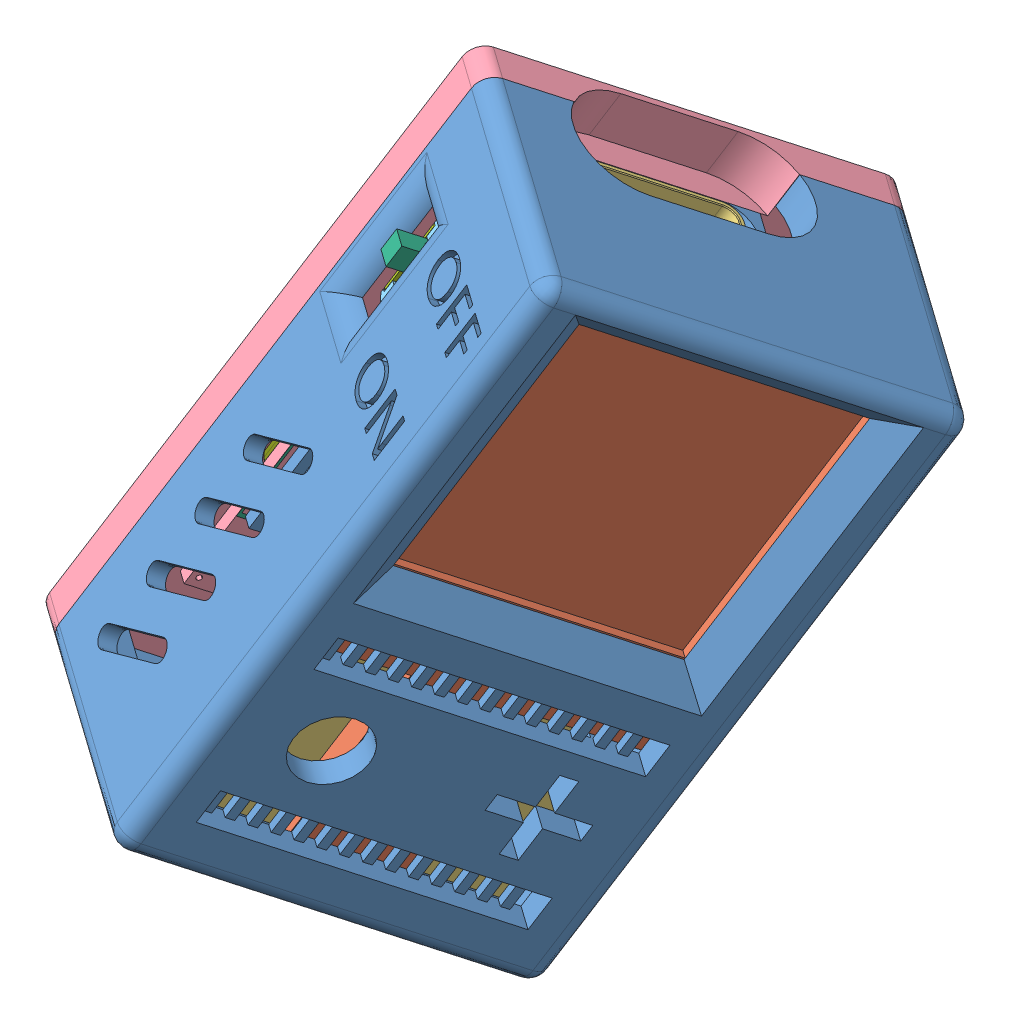
SolidWorks assembly 装配结果, configuration 默认. Lengths in mm.
Overall size (36.13 44.31 38.46).
66 component instances, 24 part files, 16 mates.
Components (placement in the parent):
- 底壳-1: 底壳 [默认] at (-149.4728 -161.4638 86.1808) x (-0.386865 -0.850817 0.355593) z (0.40861 -0.50386 -0.761028) size (36 13.58 22.5)
- 屏幕-1: 屏幕 [默认] at (-121.0492 -113.9961 50.2807) x (0.40861 -0.50386 -0.761028) z (-0.386865 -0.850817 0.355593) size (17.6 9.86 34.5)
- 电池2-1: 电池2 [默认] at (-129.898 -131.9276 58.8345) x (0.40861 -0.50386 -0.761028) z (-0.826664 0.149116 -0.542578) size (20 33.5 4.2)
- 盖子2-1: 盖子2 [默认] at (-200.8772 -117.2921 151.6108) x (-0.40861 0.50386 0.761028) z (-0.826664 0.149116 -0.542578) size (22.5 36 4.86)
- 3D_生产板_1_2025-09-30.step-1: 3D_生产板_1_2025-09-30.step [默认] at (-117.6719 -106.3839 35.2086) x (-0.40861 0.50386 0.761028) z (-0.826664 0.149116 -0.542578) size (25.17 25.38 6.33)
  - SW5~SW-SMD_MSK12CO2~SW-SMD_MSK12CO2~KENi.step-1: SW5~SW-SMD_MSK12CO2~SW-SMD_MSK12CO2~KENi.step [默认] at (16.0652 -14.3822 0.7999) x (0 1 0) z (0 0 1) size (6 5.15 1.9)
    - SW-SMD_MSK12CO2~SW-SMD_MSK12CO2~KENi.step-1: SW-SMD_MSK12CO2~SW-SMD_MSK12CO2~KENi.step [默认] at origin size (5 3.65 1.9)
    - SW-SMD_MSK12CO2~SW-SMD_MSK12CO2~KENi-0.step-1: SW-SMD_MSK12CO2~SW-SMD_MSK12CO2~KENi-0.step [默认] at origin size (1.3 2.24 1.1)
    - SW-SMD_MSK12CO2~SW-SMD_MSK12CO2~KENi-1.step-1: SW-SMD_MSK12CO2~SW-SMD_MSK12CO2~KENi-1.step [默认] at origin size (6 2.75 1.4)
  - R58~R0603~R0603~KENi.step-1: R58~R0603~R0603~KENi.step [默认] at (11.3222 -16.7282 0.7999) size (1.62 0.81 0.45)
    - R0603~R0603~KENi.step-1: R0603~R0603~KENi.step [默认] at origin size (1.62 0.81 0.45)
  - R58~R0603~R0603~KENi.step-2: R58~R0603~R0603~KENi.step [默认] at (3.7741 -26.5714 0.7999) x (0 -1 0) z (0 0 1) size (1.62 0.81 0.45)
    - R0603~R0603~KENi.step-1: R0603~R0603~KENi.step [默认] at origin size (1.62 0.81 0.45)
  - R58~R0603~R0603~KENi.step-3: R58~R0603~R0603~KENi.step [默认] at (6.1401 -27.6421 0.7999) x (-1 0 0) z (0 0 1) size (1.62 0.81 0.45)
    - R0603~R0603~KENi.step-1: R0603~R0603~KENi.step [默认] at origin size (1.62 0.81 0.45)
  - R58~R0603~R0603~KENi.step-4: R58~R0603~R0603~KENi.step [默认] at (6.1201 -26.0104 0.7999) size (1.62 0.81 0.45)
    - R0603~R0603~KENi.step-1: R0603~R0603~KENi.step [默认] at origin size (1.62 0.81 0.45)
  - R58~R0603~R0603~KENi.step-5: R58~R0603~R0603~KENi.step [默认] at (1.173 -22.5423 0.7999) x (0 -1 0) z (0 0 1) size (1.62 0.81 0.45)
    - R0603~R0603~KENi.step-1: R0603~R0603~KENi.step [默认] at origin size (1.62 0.81 0.45)
  - R58~R0603~R0603~KENi.step-6: R58~R0603~R0603~KENi.step [默认] at (8.4151 -26.9284 0.7999) x (0 1 0) z (0 0 1) size (1.62 0.81 0.45)
    - R0603~R0603~KENi.step-1: R0603~R0603~KENi.step [默认] at origin size (1.62 0.81 0.45)
  - R58~R0603~R0603~KENi.step-7: R58~R0603~R0603~KENi.step [默认] at (11.1182 -27.0814 0.7999) x (0 -1 0) z (0 0 1) size (1.62 0.81 0.45)
    - R0603~R0603~KENi.step-1: R0603~R0603~KENi.step [默认] at origin size (1.62 0.81 0.45)
  - R58~R0603~R0603~KENi.step-8: R58~R0603~R0603~KENi.step [默认] at (6.0414 -16.6772 0.7999) x (-1 0 0) z (0 0 1) size (1.62 0.81 0.45)
    - R0603~R0603~KENi.step-1: R0603~R0603~KENi.step [默认] at origin size (1.62 0.81 0.45)
  - U5~SOT-23-3_L2.9-W1.6-P1.90-LS2.8-BR~SOT-23-3L_L2.9-W1.6-H1.1-LS2.8-P0.95~KENi.step-1: U5~SOT-23-3_L2.9-W1.6-P1.90-LS2.8-BR~SOT-23-3L_L2.9-W1.6-H1.1-LS2.8-P0.95~KENi.step [默认] at (14.6372 -31.0085 0.7999) x (0 -1 0) z (0 0 1) size (2.7 2.8 1.06)
    - SOT-23-3_L2.9-W1.6-P1.90-LS2.8-BR~SOT-23-3L_L2.9-W1.6-H1.1-LS2.8-P0.95~KENi.step-1: SOT-23-3_L2.9-W1.6-P1.90-LS2.8-BR~SOT-23-3L_L2.9-W1.6-H1.1-LS2.8-P0.95~KENi.step [默认] at origin size (2.7 2.8 1.06)
  - C2~C0603~C0603_L1.6-W0.8-H0.8~KENi.step-1: C2~C0603~C0603_L1.6-W0.8-H0.8~KENi.step [默认] at (17.1363 -31.0085 0.7999) x (0 1 0) z (0 0 1) size (1.6 0.8 0.8)
    - C0603~C0603_L1.6-W0.8-H0.8~KENi.step-1: C0603~C0603_L1.6-W0.8-H0.8~KENi.step [默认] at origin size (1.6 0.8 0.8)
  - C2~C0603~C0603_L1.6-W0.8-H0.8~KENi.step-2: C2~C0603~C0603_L1.6-W0.8-H0.8~KENi.step [默认] at (16.3712 -28.5604 0.7999) x (-1 0 0) z (0 0 1) size (1.6 0.8 0.8)
    - C0603~C0603_L1.6-W0.8-H0.8~KENi.step-1: C0603~C0603_L1.6-W0.8-H0.8~KENi.step [默认] at origin size (1.6 0.8 0.8)
  - C2~C0603~C0603_L1.6-W0.8-H0.8~KENi.step-3: C2~C0603~C0603_L1.6-W0.8-H0.8~KENi.step [默认] at (4.6921 -24.1234 0.7999) x (-1 0 0) z (0 0 1) size (1.6 0.8 0.8)
    - C0603~C0603_L1.6-W0.8-H0.8~KENi.step-1: C0603~C0603_L1.6-W0.8-H0.8~KENi.step [默认] at origin size (1.6 0.8 0.8)
  - C2~C0603~C0603_L1.6-W0.8-H0.8~KENi.step-4: C2~C0603~C0603_L1.6-W0.8-H0.8~KENi.step [默认] at (16.5752 -19.0743 0.7999) size (1.6 0.8 0.8)
    - C0603~C0603_L1.6-W0.8-H0.8~KENi.step-1: C0603~C0603_L1.6-W0.8-H0.8~KENi.step [默认] at origin size (1.6 0.8 0.8)
  - C2~C0603~C0603_L1.6-W0.8-H0.8~KENi.step-5: C2~C0603~C0603_L1.6-W0.8-H0.8~KENi.step [默认] at (16.6639 -20.736 0.7999) size (1.6 0.8 0.8)
    - C0603~C0603_L1.6-W0.8-H0.8~KENi.step-1: C0603~C0603_L1.6-W0.8-H0.8~KENi.step [默认] at origin size (1.6 0.8 0.8)
  - C2~C0603~C0603_L1.6-W0.8-H0.8~KENi.step-6: C2~C0603~C0603_L1.6-W0.8-H0.8~KENi.step [默认] at (16.621 -22.5399 0.7999) x (-1 0 0) z (0 0 1) size (1.6 0.8 0.8)
    - C0603~C0603_L1.6-W0.8-H0.8~KENi.step-1: C0603~C0603_L1.6-W0.8-H0.8~KENi.step [默认] at origin size (1.6 0.8 0.8)
  - C2~C0603~C0603_L1.6-W0.8-H0.8~KENi.step-7: C2~C0603~C0603_L1.6-W0.8-H0.8~KENi.step [默认] at (6.9871 -22.6443 0.7999) x (0 1 0) z (0 0 1) size (1.6 0.8 0.8)
    - C0603~C0603_L1.6-W0.8-H0.8~KENi.step-1: C0603~C0603_L1.6-W0.8-H0.8~KENi.step [默认] at origin size (1.6 0.8 0.8)
  - U1~OLIMEX_IC-FP_TSSOP20_Pitch-0.65mm_6.6x4.5x1.2mm~TSSOP-20_L6.5-W4.4-P0.65-LS6.4-BL-EP-4~KENi.step-1: U1~OLIMEX_IC-FP_TSSOP20_Pitch-0.65mm_6.6x4.5x1.2mm~TSSOP-20_L6.5-W4.4-P0.65-LS6.4-BL-EP-4~KENi.step [默认] at (11.5772 -21.3693 0.7999) x (-1 0 0) z (0 0 1) size (6.5 6.4 1.2)
    - OLIMEX_IC-FP_TSSOP20_Pitch-0.65mm_6.6x4.5x1.2mm~TSSOP-20_L6.5-W4.4-P0.65-LS6.4-BL-EP-4~KENi.step-1: OLIMEX_IC-FP_TSSOP20_Pitch-0.65mm_6.6x4.5x1.2mm~TSSOP-20_L6.5-W4.4-P0.65-LS6.4-BL-EP-4~KENi.step [默认] at origin size (6.5 6.4 1.2)
  - D7~SOD-323F_L1.7-W1.3-LS2.5-R-RD-1~SOD-323F_L1.7-W1.3-LS2.5-RD~KENi.step-1: D7~SOD-323F_L1.7-W1.3-LS2.5-R-RD-1~SOD-323F_L1.7-W1.3-LS2.5-RD~KENi.step [默认] at (13.5152 -27.1834 0.7999) x (0 1 0) z (0 0 1) size (2.5 1.25 0.66)
    - SOD-323F_L1.7-W1.3-LS2.5-R-RD-1~SOD-323F_L1.7-W1.3-LS2.5-RD~KENi.step-1: SOD-323F_L1.7-W1.3-LS2.5-R-RD-1~SOD-323F_L1.7-W1.3-LS2.5-RD~KENi.step [默认] at origin size (2.5 1.25 0.66)
  - U29~CONN-SMD_2P-P1.00_CS-1254R-02~CONN-SMD_2P-P1.00_CS-1254R-02~KENi.step-1: U29~CONN-SMD_2P-P1.00_CS-1254R-02~CONN-SMD_2P-P1.00_CS-1254R-02~KENi.step [默认] at (0.51 -30.0904 0.7999) size (4.01 5.05 3.15)
    - CONN-SMD_2P-P1.00_CS-1254R-02~CONN-SMD_2P-P1.00_CS-1254R-02~KENi.step-1: CONN-SMD_2P-P1.00_CS-1254R-02~CONN-SMD_2P-P1.00_CS-1254R-02~KENi.step [默认] at origin size (4.01 5.05 3.15)
  - D8~SOD-323_L1.7-W1.3-LS2.6-RD-1~SOD-323_L1.7-W1.3-LS2.6-RD-1~KENi.step-1: D8~SOD-323_L1.7-W1.3-LS2.6-RD-1~SOD-323_L1.7-W1.3-LS2.6-RD-1~KENi.step [默认] at (6.9871 -19.4823 0.7999) x (0 -1 0) z (0 0 1) size (2.55 1.25 1.05)
    - SOD-323_L1.7-W1.3-LS2.6-RD-1~SOD-323_L1.7-W1.3-LS2.6-RD-1~KENi.step-1: SOD-323_L1.7-W1.3-LS2.6-RD-1~SOD-323_L1.7-W1.3-LS2.6-RD-1~KENi.step [默认] at origin size (2.55 1.25 1.05)
  - SW4~SW-SMD_TM-2024A~SW-SMD_TM-2024A~KENi.step-1: SW4~SW-SMD_TM-2024A~SW-SMD_TM-2024A~KENi.step [默认] at (0.765 -14.5862 0.7999) x (0 1 0) z (0 0 1) size (13.16 9 2.8)
    - SW-SMD_TM-2024A~SW-SMD_TM-2024A~KENi.step-1: SW-SMD_TM-2024A~SW-SMD_TM-2024A~KENi.step [默认] at origin size (13.16 9 2.8)
  - Q6~SOT-23_L2.9-W1.3-P0.95-LS2.4-BR~SOT-23-3P~KENi.step-1: Q6~SOT-23_L2.9-W1.3-P0.95-LS2.4-BR~SOT-23-3P~KENi.step [默认] at (16.4222 -25.8574 0.7999) x (0 -1 0) z (0 0 1) size (2.51 2.9 1.05)
    - SOT-23_L2.9-W1.3-P0.95-LS2.4-BR~SOT-23-3P~KENi.step-1: SOT-23_L2.9-W1.3-P0.95-LS2.4-BR~SOT-23-3P~KENi.step [默认] at origin size (2.51 2.9 1.05)
  - U25~SOT-23-3_L2.9-W1.3-P1.90-LS2.4-BR~SOT-23-3P_L2.9-W1.3-H1.0-LS2.4-P0.95~KENi.step-1: U25~SOT-23-3_L2.9-W1.3-P1.90-LS2.4-BR~SOT-23-3P_L2.9-W1.3-H1.0-LS2.4-P0.95~KENi.step [默认] at (1.122 -25.7044 0.7999) size (2.5 2.89 1.05)
    - SOT-23-3_L2.9-W1.3-P1.90-LS2.4-BR~SOT-23-3P_L2.9-W1.3-H1.0-LS2.4-P0.95~KENi.step-1: SOT-23-3_L2.9-W1.3-P1.90-LS2.4-BR~SOT-23-3P_L2.9-W1.3-H1.0-LS2.4-P0.95~KENi.step [默认] at origin size (2.5 2.89 1.05)
  - U37~SOT-23-6_L2.9-W1.6-P0.95-LS2.8-BL~SOT-23-6_L2.9-W1.6-H1.5-LS2.8-P0.95~KENi.step-1: U37~SOT-23-6_L2.9-W1.6-P0.95-LS2.8-BL~SOT-23-6_L2.9-W1.6-H1.5-LS2.8-P0.95~KENi.step [默认] at (4.1311 -21.5733 0.7999) x (0 1 0) z (0 0 1) size (2.88 2.79 1.64)
    - SOT-23-6_L2.9-W1.6-P0.95-LS2.8-BL~SOT-23-6_L2.9-W1.6-H1.5-LS2.8-P0.95~KENi.step-1: SOT-23-6_L2.9-W1.6-P0.95-LS2.8-BL~SOT-23-6_L2.9-W1.6-H1.5-LS2.8-P0.95~KENi.step [默认] at origin size (2.88 2.79 1.64)
  - U24~SX1278~COMM-SMD_SX1278ZTR4-GC~KENi.step-1: U24~SX1278~COMM-SMD_SX1278ZTR4-GC~KENi.step [默认] at (9.525 -20.447 0) x (-1 0 0) z (0 0 -1) size (16.5 16.5 2.33)
    - SX1278~COMM-SMD_SX1278ZTR4-GC~KENi.step-1: SX1278~COMM-SMD_SX1278ZTR4-GC~KENi.step [默认] at origin size (16.5 16.5 2.33)
  - FPC1~FPC-SMD_12P-P0.50_THD0509-12CL-GF~FPC-SMD_12P-P0.50_THD0509-12CL-GF~KENi.step-1: FPC1~FPC-SMD_12P-P0.50_THD0509-12CL-GF~FPC-SMD_12P-P0.50_THD0509-12CL-GF~KENi.step [默认] at (7.875 -31.0085 0.7999) size (8 3.8 1)
    - FPC-SMD_12P-P0.50_THD0509-12CL-GF~FPC-SMD_12P-P0.50_THD0509-12CL-GF~KENi.step-1: FPC-SMD_12P-P0.50_THD0509-12CL-GF~FPC-SMD_12P-P0.50_THD0509-12CL-GF~KENi.step [默认] at origin size (8 3.8 1)
  - USB2~USB-C-SMD_TYPE-C16PIN~USB-C-SMD_TYPE-C16PIN-SHOUHAN~KENi.step-1: USB2~USB-C-SMD_TYPE-C16PIN~USB-C-SMD_TYPE-C16PIN-SHOUHAN~KENi.step [默认] at (8.6698 -12.6992 0.7999) x (-1 0 0) z (0 0 1) size (8.95 7.9 4.2)
    - USB-C-SMD_TYPE-C16PIN~USB-C-SMD_TYPE-C16PIN-SHOUHAN~KENi.step-1: USB-C-SMD_TYPE-C16PIN~USB-C-SMD_TYPE-C16PIN-SHOUHAN~KENi.step [默认] at origin size (8.95 7.9 4.2)
  - Board~KENi.step-1: Board~KENi.step [默认] at origin size (20.37 24 0.8)
  - TopSilkscreen~KENi.step-1: TopSilkscreen~KENi.step [默认] at (0 0 0.8199) size (20.37 23.79 0.04)
  - BottomSilkscreen~KENi.step-1: BottomSilkscreen~KENi.step [默认] at (0 0 -0.02) size (20 23.06 0.01)
Mates (geometry in assembly coordinates):
- 重合24: coincident: line of 底壳-1 through (-120.0445 -126.878 48.0848) axis (0.386865 0.850817 -0.355593); plane of 屏幕-1 through (-114.5388 -113.786 42.3729) normal (-0.40861 0.50386 0.761028)
- 重合26: coincident: line of 底壳-1 through (-114.1255 -113.8605 42.6442) axis (-0.40861 0.50386 0.761028); plane of 屏幕-1 through (-120.7538 -106.1222 53.9482) normal (-0.386865 -0.850817 0.355593)
- 重合37: coincident anti-aligned: plane of 底壳-1 through (-150.7128 -161.2401 85.3669) normal (-0.826664 0.149116 -0.542578); plane of 屏幕-1 through (-119.7596 -114.2287 51.1271) normal (0.826664 -0.149116 0.542578)
- 重合58: coincident: plane of 底壳-1 through (-121.655 -111.7687 32.427) normal (0.40861 -0.50386 -0.761028); line of 盖子-1 through (-123.365 -114.8135 28.9059) axis (-0.386865 -0.850817 0.355593)
- 重合78: coincident anti-aligned: plane of 底壳-1 through (-125.6713 -134.2205 41.8306) normal (-0.40861 0.50386 0.761028); plane of 电池-1 through (-128.3264 -142.027 45.5735) normal (0.40861 -0.50386 -0.761028)
- 重合79: coincident anti-aligned: plane of 底壳-1 through (-155.6314 -160.3529 82.1386) normal (-0.826664 0.149116 -0.542578); plane of 电池-1 through (-130.5527 -133.8401 51.2155) normal (0.826664 -0.149116 0.542578)
- 重合80: coincident anti-aligned: plane of 底壳-1 through (-126.0799 -133.7167 42.5916) normal (-0.386865 -0.850817 0.355593); plane of 电池-1 through (-124.0709 -132.668 41.662) normal (0.386865 0.850817 -0.355593)
- 重合105: coincident anti-aligned: plane of 底壳-1 through (-113.7044 -113.6933 39.2841) normal (-0.40861 0.50386 0.761028); plane of 电池2-1 through (-130.186 -141.5605 48.885) normal (0.40861 -0.50386 -0.761028)
- 重合100: coincident anti-aligned: plane of 底壳-1 through (-160.6989 -159.4388 78.8126) normal (-0.826664 0.149116 -0.542578); plane of 盖子2-1 through (-200.8772 -117.2921 151.6108) normal (0.826664 -0.149116 0.542578)
- 重合101: coincident aligned: plane of 底壳-1 through (-121.655 -111.7687 32.427) normal (0.40861 -0.50386 -0.761028); plane of 盖子2-1 through (-123.3084 -111.4705 31.3418) normal (0.40861 -0.50386 -0.761028)
- 重合102: coincident aligned: plane of 底壳-1 through (-135.5822 -142.3981 45.2283) normal (-0.386865 -0.850817 0.355593); plane of 盖子2-1 through (-146.4292 -130.763 61.2663) normal (-0.386865 -0.850817 0.355593)
- 重合106: coincident anti-aligned: plane of 底壳-1 through (-122.0809 -103.3642 54.8851) normal (-0.386865 -0.850817 0.355593); plane of 电池2-1 through (-125.3982 -102.9809 52.1932) normal (0.386865 0.850817 -0.355593)
- 重合108: coincident anti-aligned: plane of 屏幕-1 through (-121.0492 -113.9961 50.2807) normal (-0.826664 0.149116 -0.542578); plane of 电池2-1 through (-129.898 -131.9276 58.8345) normal (0.826664 -0.149116 0.542578)
- 重合130: coincident anti-aligned: plane of 电池2-1 through (-133.37 -131.3014 56.5556) normal (-0.826664 0.149116 -0.542578); plane of 3D_生产板_1_2025-09-30.step-1/U24~SX1278~COMM-SMD_SX1278ZTR4-GC~KENi.step-1/SX1278~COMM-SMD_SX1278ZTR4-GC~KENi.step-1 through (-127.5555 -119.3274 50.9875) normal (0.826664 -0.149116 0.542578)
- 重合131: coincident anti-aligned: plane of 底壳-1 through (-113.7044 -113.6933 39.2841) normal (-0.40861 0.50386 0.761028); plane of 3D_生产板_1_2025-09-30.step-1/Board~KENi.step-1 through (-129.5893 -135.6824 45.3137) normal (0.40861 -0.50386 -0.761028)
- 重合132: coincident anti-aligned: plane of 底壳-1 through (-123.1378 -106.5493 54.551) normal (-0.386865 -0.850817 0.355593); plane of 3D_生产板_1_2025-09-30.step-1/Board~KENi.step-1 through (-120.3053 -115.2644 36.7801) normal (0.386865 0.850817 -0.355593)
